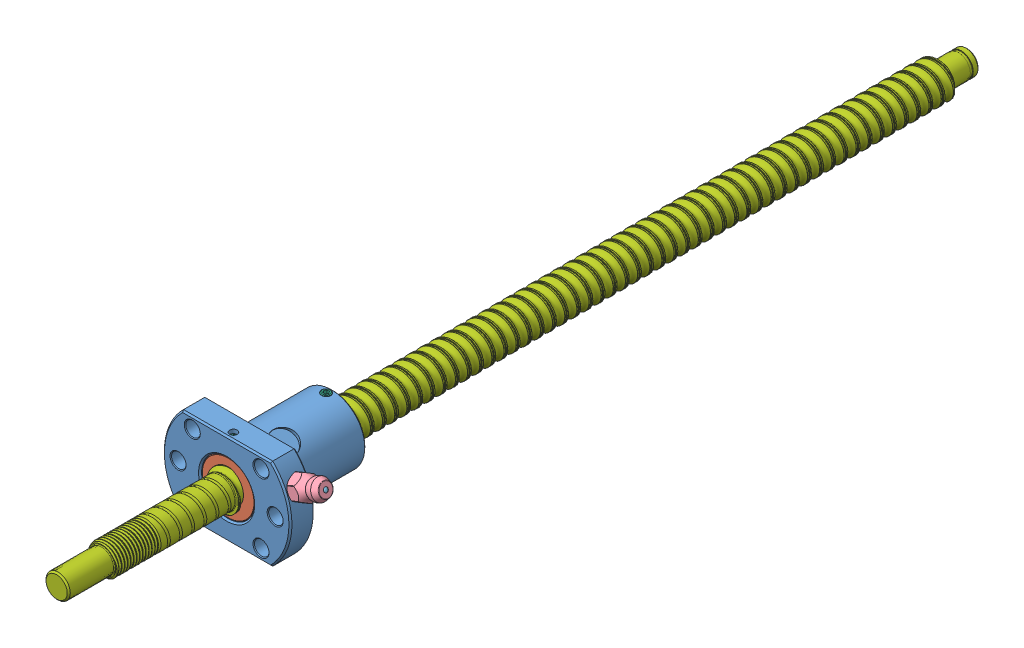
SolidWorks assembly SFU1204-300 With Nut, configuration Default. Lengths in mm.
Overall size (51.14 30.68 300).
12 component instances, 7 part files, 2 mates.
Components (placement in the parent):
- SFU1204-3-1: SFU1204-3 [Default] at origin size (51.14 30.68 39.46)
  - SFU Ball Nut-1: SFU Ball Nut [1204-3] at origin size (42 30 35)
  - SFU1204 Washer Front-1: SFU1204 Washer Front [Default] at origin size (17.5 17.5 9.46)
  - SFU1204 Washer Back-1: SFU1204 Washer Back [Default] at origin size (17.5 17.5 9.46)
  - Grease Nipple A M6x1.00-2: Grease Nipple A M6x1.00 [Default] at (26.2888 10.8892 -4.25) x (0.382683 -0.92388 0) z (0 0 1) size (8.34 16.1 7)
    - Grease Nipple A-1: Grease Nipple A [A M6x1.00] at origin size (8.34 16 7)
    - Steel Ball-1: Steel Ball [Ø 2.50] at (0 1.1952 0) size (2.5 2.5 2.5)
  - socket set screw cone point_iso-1: socket set screw cone point_iso [ISO 4027 - M3 x 5-C] at (0 13.75 -2.25) x (0 -1 0) z (-1 0 0) size (5 3 3)
  - socket set screw cone point_iso-2: socket set screw cone point_iso [ISO 4027 - M3 x 5-C] at (0 -13.75 -2.25) x (0 1 0) z (-1 0 0) size (5 3 3)
  - socket set screw cone point_iso-3: socket set screw cone point_iso [ISO 4027 - M3 x 2.5-C] at (0 11.25 -32.75) x (0 -1 0) z (1 0 0) size (2.5 3 3)
  - socket set screw cone point_iso-4: socket set screw cone point_iso [ISO 4027 - M3 x 2.5-C] at (0 -11.25 -32.75) x (0 1 0) z (1 0 0) size (2.5 3 3)
- SFU1204-300-1: SFU1204-300 [1204-300] at (0 0 56) size (12.18 12.18 300)
Mates (geometry in assembly coordinates):
- Screw: screw = 4 mm aligned: cylinder of SFU1204-3-1/SFU Ball Nut-1 through (0 0 0) axis (0 0 1) radius 11; cylinder of SFU1204-300-1 through (0 0 2) axis (0 0 1) radius 5
- Distance: distance = 56 mm aligned: plane of SFU1204-300-1 through (0 0 56) normal (0 0 1); plane of SFU1204-3-1/SFU Ball Nut-1 through (8.75 0 0) normal (0 0 1)
